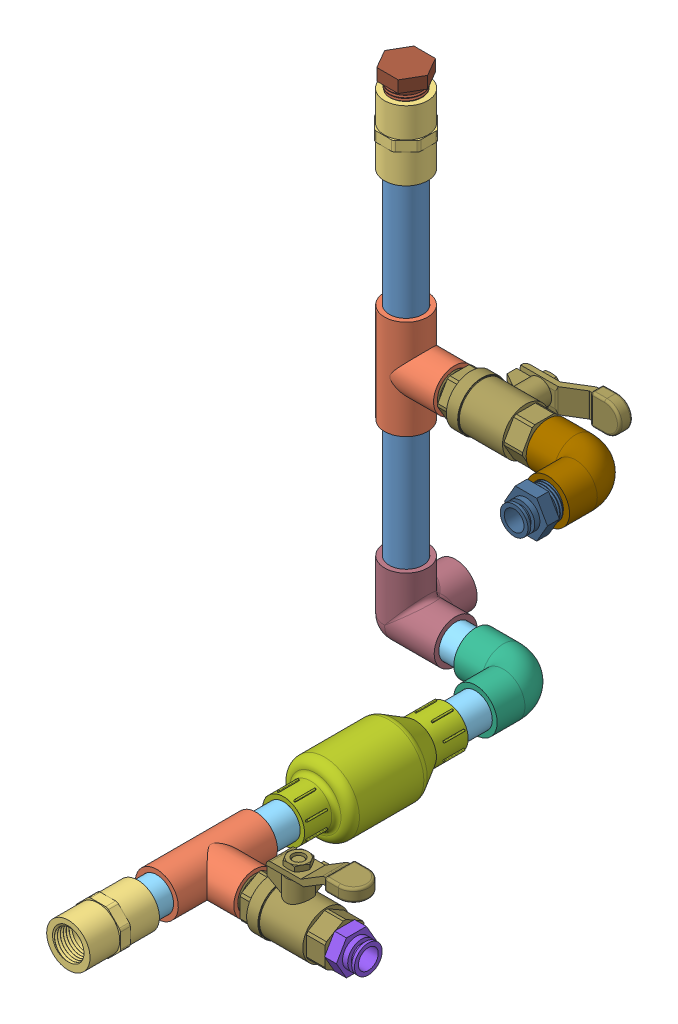
SolidWorks assembly manifold_intake, configuration Default. Lengths in mm.
Overall size (195.82 327.41 334.64).
20 component instances, 13 part files, 70 mates.
Components (placement in the parent):
- pvc-050-0045-1: pvc-050-0045 [Default] at (13.1169 27.275 86.4941) size (21.34 114.3 21.34)
- threaded_tee-1: threaded_tee [4880K392] at (13.1169 153.767 86.4941) x (0 -1 0) z (0 0 1) size (63.5 45.17 27.56)
- pvc-050-0045-2: pvc-050-0045 [Default] at (13.1169 165.959 86.4941) size (21.34 114.3 21.34)
- new adapter-1: new adapter [Default] at (13.1169 305.659 86.4941) x (0.071121 0 -0.997468) z (0 1 0) size (29.21 29.21 45.39)
- TRUE_NIPPLE-1: TRUE_NIPPLE [4830K171] at (102.7698 153.767 86.4941) size (28.84 22.41 22.44)
- pvc-050-0015-1: pvc-050-0015 [Default] at (76.6169 14.575 86.4941) x (0 -0.826891 0.562362) z (0 -0.562362 -0.826891) size (21.34 50.8 21.34)
- unthreaded 90-1: unthreaded 90 [Default] at (89.3169 14.575 118.2441) x (0 1 0) z (0 0 1) size (27.78 45.64 45.64)
- pvc-050-0015-2: pvc-050-0015 [Default] at (89.3169 14.575 149.9941) x (1 0 0) z (0 1 0) size (21.34 50.8 21.34)
- BACKFLOW-1: BACKFLOW [46835K52] at (89.3169 14.575 188.8256) size (44.7 44.7 104.77)
- pvc-050-0015-3: pvc-050-0015 [Default] at (89.3169 14.575 278.4572) x (1 0 0) z (0 1 0) size (21.34 50.8 21.34)
- new adapter-2: new adapter [Default] at (89.3169 14.575 379.0412) x (0.071121 0.997468 0) z (0 0 1) size (29.21 29.21 45.39)
- threaded_tee-2: threaded_tee [4880K392] at (89.3169 14.575 290.6492) x (0 0 -1) z (0 -1 0) size (63.5 45.17 27.56)
- pvc-050-0015-4: pvc-050-0015 [Default] at (89.3169 14.575 302.8412) x (0 1 0) z (1 0 0) size (21.34 50.8 21.34)
- connector_orange-1: connector_orange [Default] at (177.8359 14.575 290.6492) x (0 -0.866025 -0.5) z (0 -0.5 0.866025) size (25.66 23.29 22.23)
- double thread-1: double thread [Default] at (135.6537 153.767 118.2441) x (0 1 0) z (0 0 1) size (27.78 46.58 46.58)
- backflow_inlet-1: backflow_inlet [Default] at (135.6537 153.767 124.5941) x (-0.5 -0.866025 0) z (-0.866025 0.5 0) size (27.5 33.02 23.81)
- cap-1: cap [Default] at (13.1169 312.009 86.4941) size (27.5 25.4 23.81)
- short valve-1: short valve [47865K13] at (72.1465 153.767 86.4941) x (0 1 0) z (-1 0 0) size (31.24 56.77 85.34)
- side-outlet-elbow-2: side-outlet-elbow [4880K631] at (13.1169 14.575 86.4941) x (-1 0 0) z (0 0 -1) size (45.53 45.53 45.53)
- short valve-2: short valve [47865K13] at (148.3465 14.575 290.6492) x (0 0 1) z (-1 0 0) size (31.24 56.77 85.34)
Mates (geometry in assembly coordinates):
- Concentric1: concentric: circle of pvc-050-0045-1; circle of threaded_tee-1
- Parallel1: parallel: plane of threaded_tee-1 through (44.1049 140.3304 86.4941) normal (1 0 0); plane of assembly through (0 0 0) normal (1 0 0)
- Coincident2: coincident: plane of pvc-050-0045-1 through (13.1169 141.575 86.4941) normal (0 1 0); plane of threaded_tee-1 through (13.1169 141.575 86.4941) normal (0 -1 0)
- Concentric2: concentric: circle of threaded_tee-1; circle of pvc-050-0045-2
- Coincident3: coincident: plane of threaded_tee-1 through (13.1169 165.959 86.4941) normal (0 1 0); plane of pvc-050-0045-2 through (13.1169 165.959 86.4941) normal (0 -1 0)
- Concentric3: concentric: circle of pvc-050-0045-2; circle of new adapter-1
- Parallel2: parallel: plane of new adapter-1 through (-1.1706 286.609 92.4122) normal (-1 0 0); plane of assembly through (0 0 0) normal (1 0 0)
- Coincident5: coincident: plane of pvc-050-0045-2 through (13.1169 280.259 86.4941) normal (0 1 0); plane of new adapter-1 through (13.1169 280.259 86.4941) normal (0 -1 0)
- Concentric4: concentric: circle of pvc-050-0045-1; circle of side-outlet-elbow-2
- Parallel3: parallel: plane of threaded_tee-1 through (44.1049 140.3304 86.4941) normal (1 0 0); plane of side-outlet-elbow-2 through (44.8669 14.575 86.4941) normal (1 0 0)
- Coincident7: coincident: plane of pvc-050-0045-1 through (13.1169 27.275 86.4941) normal (0 -1 0); plane of side-outlet-elbow-2 through (5.2175 27.275 86.4941) normal (0 1 0)
- Coincident10: coincident: plane of side-outlet-elbow-2 through (25.8169 6.6756 86.4941) normal (1 0 0); plane of pvc-050-0015-1 through (25.8169 14.575 86.4941) normal (-1 0 0)
- Concentric6: concentric: circle of side-outlet-elbow-2; circle of pvc-050-0015-1
- Coincident12: coincident: plane of pvc-050-0015-1 through (76.6169 14.575 86.4941) normal (1 0 0); plane of unthreaded 90-1 through (76.6169 14.575 86.4941) normal (-1 0 0)
- Concentric8: concentric: circle of pvc-050-0015-1; circle of unthreaded 90-1
- Perpendicular1: perpendicular: plane of side-outlet-elbow-2 through (-0.6626 46.325 86.4941) normal (0 1 0); plane of unthreaded 90-1 through (89.3169 14.575 118.2441) normal (0 0 1)
- Concentric9: concentric: circle of unthreaded 90-1; circle of pvc-050-0015-2
- Coincident14: coincident: plane of unthreaded 90-1 through (89.3169 14.575 99.1941) normal (0 0 1); plane of pvc-050-0015-2 through (89.3169 14.575 99.1941) normal (0 0 -1)
- Coincident15: coincident: plane of pvc-050-0015-2 through (89.3169 14.575 149.9941) normal (0 0 1); plane of BACKFLOW-1 through (89.3169 25.243 149.9941) normal (0 0 -1)
- Coincident17: coincident: plane of pvc-050-0015-2 through (89.3169 14.575 149.9941) normal (0 0 1); plane of BACKFLOW-1 through (89.3169 25.243 149.9941) normal (0 0 -1)
- Concentric10: concentric: circle of pvc-050-0015-2; cylinder of BACKFLOW-1 through (89.3169 14.575 241.2131) axis (0 0 1) radius 10.668
- Concentric11: concentric: circle of BACKFLOW-1; circle of pvc-050-0015-3
- Coincident19: coincident: plane of BACKFLOW-1 through (89.3169 25.243 227.6572) normal (0 0 1); plane of pvc-050-0015-3 through (89.3169 14.575 227.6572) normal (0 0 -1)
- Concentric12: concentric: circle of pvc-050-0015-3; circle of new adapter-2
- Concentric13: concentric: circle of pvc-050-0015-3; circle of threaded_tee-2
- Coincident20: coincident: plane of pvc-050-0015-3 through (89.3169 14.575 278.4572) normal (0 0 1); plane of threaded_tee-2 through (89.3169 14.575 278.4572) normal (0 0 -1)
- Parallel4: parallel: plane of side-outlet-elbow-2 through (44.8669 14.575 86.4941) normal (1 0 0); plane of threaded_tee-2 through (120.3049 14.575 277.2126) normal (1 0 0)
- Concentric14: concentric: circle of threaded_tee-2; circle of pvc-050-0015-4
- Coincident22: coincident: plane of threaded_tee-2 through (89.3169 14.575 302.8412) normal (0 0 1); plane of pvc-050-0015-4 through (89.3169 14.575 302.8412) normal (0 0 -1)
- Coincident23: coincident: plane of new adapter-2 through (89.3169 14.575 353.6412) normal (0 0 -1); plane of pvc-050-0015-4 through (89.3169 14.575 353.6412) normal (0 0 1)
- Concentric15: concentric: circle of threaded_tee-2; cylinder of ? through (107.0195 14.575 290.6492) axis (1 0 0) radius 7.8994
- Coincident24: coincident: plane of threaded_tee-2 through (120.3049 14.575 277.2126) normal (1 0 0); plane of ? through (120.3049 14.575 290.6492) normal (-1 0 0)
- Concentric16: concentric: circle of threaded_tee-1; circle of ?
- Coincident26: coincident: plane of TRUE_NIPPLE-1 through (49.5477 153.767 86.4941) normal (1 0 0); plane of ? through (49.5477 153.767 86.4941) normal (-1 0 0)
- Concentric17: concentric: circle of ?; cylinder of ? through (94.9999 153.767 86.4941) axis (1 0 0) radius 7.8994
- Coincident27: coincident: plane of ? through (108.2852 141.2702 79.2791) normal (1 0 0); plane of ? through (108.2852 153.767 86.4941) normal (-1 0 0)
- Concentric18: concentric: circle of threaded_tee-1; circle of ?
- Concentric19: concentric: circle of ?; circle of ?
- Parallel6: parallel: plane of side-outlet-elbow-2 through (13.1169 14.575 54.7441) normal (0 0 -1); plane of ? through (242.2258 14.575 247.6724) normal (0 0 -1)
- Coincident30: coincident: plane of ?; plane of ? through (122.5727 27.0718 283.4341) normal (-1 0 0)
- Coincident31: coincident: plane of ? through (181.3102 14.575 290.6492) normal (1 0 0); plane of ? through (181.3102 14.575 290.6492) normal (-1 0 0)
- Concentric20: concentric: circle of ?; circle of ?
- Concentric21: concentric: circle of ?; circle of connector_orange-1
- Parallel7: parallel: plane of ? through (219.4886 27.0718 297.8642) normal (0 1 0); plane of connector_orange-1 through (189.4382 25.6875 284.2334) normal (0 1 0)
- Distance2: distance = 0.508 mm: plane of ? through (181.3102 14.575 290.6492) normal (1 0 0); plane of connector_orange-1 through (181.8182 14.575 290.6492) normal (-1 0 0)
- Distance3: distance = 2.54 mm: plane of ? through (108.2852 141.2702 79.2791) normal (1 0 0); plane of double thread-1 through (110.8252 153.767 86.4941) normal (-1 0 0)
- Concentric22: concentric: circle of ?; circle of double thread-1
- Distance4: distance = 6.35 mm: plane of backflow_inlet-1 through (135.6537 153.767 124.5941) normal (0 0 -1); plane of double thread-1 through (135.6537 153.767 118.2441) normal (0 0 1)
- Concentric23: concentric: circle of double thread-1; circle of backflow_inlet-1
- Concentric24: concentric: circle of new adapter-1; circle of cap-1
- Distance5: distance = 6.35 mm: plane of cap-1 through (13.1169 312.009 86.4941) normal (0 -1 0); plane of new adapter-1 through (13.1169 305.659 86.4941) normal (0 1 0)
- Concentric26: concentric: circle of pvc-050-0045-1; circle of side-outlet-elbow-2
- Concentric27: concentric: circle of pvc-050-0015-1; circle of side-outlet-elbow-2
- Parallel8: parallel: plane of new adapter-2 through (89.3169 14.575 379.0412) normal (0 0 1); plane of side-outlet-elbow-2 through (13.1169 14.575 54.7441) normal (0 0 -1)
- Coincident34: coincident: plane of pvc-050-0045-1 through (13.1169 27.275 86.4941) normal (0 -1 0); plane of side-outlet-elbow-2 through (5.2175 27.275 86.4941) normal (0 1 0)
- Coincident35: coincident: plane of pvc-050-0015-1 through (25.8169 14.575 86.4941) normal (-1 0 0); plane of side-outlet-elbow-2 through (25.8169 6.6756 86.4941) normal (1 0 0)
- Concentric29: concentric: circle of threaded_tee-2; circle of short valve-2
- Distance8: distance = 3.175 mm: plane of threaded_tee-2 through (120.3049 14.575 277.2126) normal (1 0 0); plane of short valve-2 through (123.4799 36.2201 278.1524) normal (-1 0 0)
- Coincident42: coincident: plane of connector_orange-1 through (177.8359 14.575 290.6492) normal (-1 0 0); plane of short valve-2 through (177.8359 14.575 290.6492) normal (1 0 0)
- Concentric30: concentric: cylinder of connector_orange-1 through (193.0759 14.575 290.6492) axis (1 0 0) radius 6.35; cylinder of short valve-2 through (148.3465 14.575 290.6492) axis (1 0 0) radius 15.621
- Parallel12: parallel: plane of double thread-1 through (135.6537 153.767 118.2441) normal (0 0 1); plane of side-outlet-elbow-2 through (13.1169 14.575 54.7441) normal (0 0 -1)
- Parallel13: parallel: plane of backflow_inlet-1 through (128.7796 141.8607 132.2141) normal (0 -1 0); plane of short valve-1 through (139.8142 141.2702 79.2791) normal (0 -1 0)
- Coincident46: coincident: plane of TRUE_NIPPLE-1 through (103.9037 153.767 86.4941) normal (1 0 0); plane of double thread-1 through (103.9037 153.767 86.4941) normal (-1 0 0)
- Concentric31: concentric: circle of TRUE_NIPPLE-1; circle of double thread-1
- Concentric32: concentric: circle of threaded_tee-1; circle of short valve-1
- Distance9: distance = 3.175 mm: plane of short valve-1 through (47.2799 141.2702 64.849) normal (-1 0 0); plane of threaded_tee-1 through (44.1049 140.3304 86.4941) normal (1 0 0)
- Coincident48: coincident: plane of TRUE_NIPPLE-1 through (101.6359 153.767 86.4941) normal (-1 0 0); plane of short valve-1 through (101.6359 153.767 86.4941) normal (1 0 0)
- Concentric33: concentric: circle of TRUE_NIPPLE-1; circle of short valve-1
- Parallel15: parallel: plane of new adapter-2 through (83.3988 28.8625 359.9912) normal (0 1 0); plane of short valve-2 through (183.6144 55.723 290.6492) normal (0 1 0)
- Parallel16: parallel: plane of connector_orange-1 through (185.4559 25.6875 284.2334) normal (0 1 0); plane of short valve-2 through (183.6144 55.723 290.6492) normal (0 1 0)
